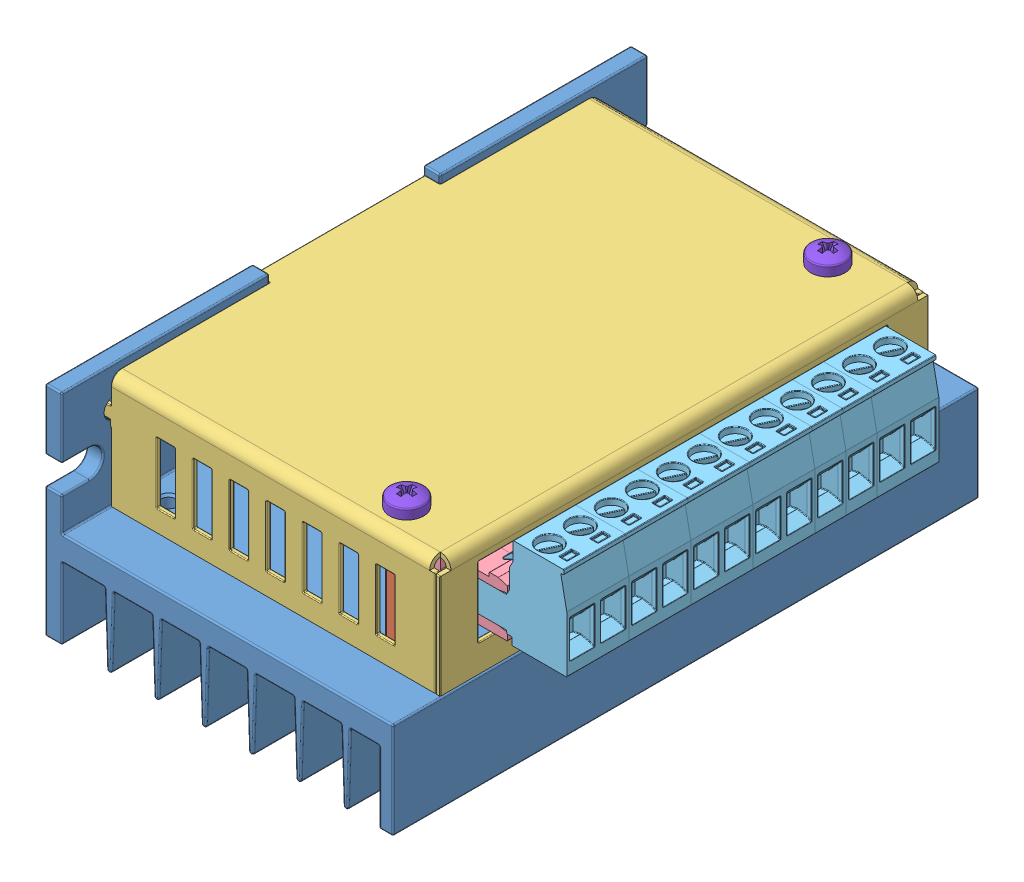
SolidWorks assembly TB6600, configuration Default. Lengths in mm.
Overall size (70.98 37.35 96).
12 component instances, 8 part files, 33 mates.
Components (placement in the parent):
- TB6600 Sink-1: TB6600 Sink [Default] at origin size (57 35.75 96)
- Distance-1: Distance [M3x18] at (43 0 -34.5) size (5 24 4.5)
- Distance-2: Distance [M3x18] at (43 0 34.5) size (5 24 4.5)
- TB6600 Cover-1: TB6600 Cover [Default] at (0 18.75 0) size (56.5 19.75 80)
- Header 200mil-1: Header 200mil [N12] at (48.5 6.85 30.96) size (12 12.2 60.96)
- Plug 200mil-2: Plug 200mil [N2] at (62.83 10.65 25.88) x (-1 0 0) z (0 0 -1) size (18.2 15 10.16)
- Plug 200mil-3: Plug 200mil [N4] at (62.83 10.65 5.56) x (-1 0 0) z (0 0 -1) size (18.2 15 20.32)
- Plug 200mil-4: Plug 200mil [N6] at (62.83 10.65 -24.92) x (-1 0 0) z (0 0 -1) size (18.2 15 30.48)
- LED 3mm Double Stand-1: LED 3mm Double Stand [Default] at (45 5.84 -31) size (11.75 10.16 4.5)
- a6fr-6101-1: a6fr-6101 [Default] at (36.4 6.2 -36.5) x (-1 0 0) z (0 0 -1) size (16.8 13.4 9.9)
- pan head cross recess screw_iso-1: pan head cross recess screw_iso [ISO 7045 - M3 x 4 - Z - 4C] at (43 21.15 -34.5) x (0 -1 0) z (0 0 -1) size (6.35 5.6 5.6)
- pan head cross recess screw_iso-2: pan head cross recess screw_iso [ISO 7045 - M3 x 4 - Z - 4C] at (43 21.15 34.5) x (0 -1 0) z (0 0 -1) size (6.35 5.6 5.6)
Mates (geometry in assembly coordinates):
- Concentric1: concentric aligned: cylinder of TB6600 Sink-1 through (43 0 -34.5) axis (0 1 0) radius 1.25; cylinder of Distance-1 through (43 -6 -34.5) axis (0 1 0) radius 1.5
- Concentric2: concentric aligned: cylinder of TB6600 Sink-1 through (43 0 34.5) axis (0 1 0) radius 1.25; cylinder of Distance-2 through (43 -6 34.5) axis (0 1 0) radius 1.5
- Coincident1: coincident: plane of TB6600 Sink-1 through (0.25 0 48) normal (0 1 0); plane of Distance-1 through (43 0 -34.5) normal (0 -1 0)
- Coincident2: coincident anti-aligned: plane of TB6600 Sink-1 through (0.25 0 48) normal (0 1 0); plane of Distance-2 through (43 0 34.5) normal (0 -1 0)
- Parallel1: parallel aligned: plane of TB6600 Sink-1 through (0 0 0) normal (1 0 0); plane of Distance-1 through (43 0 -34.5) normal (1 0 0)
- Parallel2: parallel aligned: plane of TB6600 Sink-1 through (0 0 0) normal (1 0 0); plane of Distance-2 through (43 0 34.5) normal (1 0 0)
- Concentric3: concentric aligned: cylinder of Distance-2 through (43 18 34.5) axis (0 1 0) radius 1.25; cylinder of TB6600 Cover-1 through (43 18.75 34.5) axis (0 1 0) radius 1.5
- Concentric4: concentric aligned: cylinder of Distance-1 through (43 18 -34.5) axis (0 1 0) radius 1.25; cylinder of TB6600 Cover-1 through (43 18.75 -34.5) axis (0 1 0) radius 1.5
- Coincident3: coincident anti-aligned: plane of Distance-1 through (43 18 -34.5) normal (0 1 0); plane of TB6600 Cover-1 through (53.25 18 40) normal (0 -1 0)
- Concentric5: concentric aligned: cylinder of TB6600 Cover-1 through (43 18.75 -34.5) axis (0 1 0) radius 1.5; cylinder of pan head cross recess screw_iso-1 through (43 46.55 -34.5) axis (0 1 0) radius 1.5
- Concentric6: concentric aligned: cylinder of TB6600 Cover-1 through (43 18.75 34.5) axis (0 1 0) radius 1.5; cylinder of pan head cross recess screw_iso-2 through (43 46.55 34.5) axis (0 1 0) radius 1.5
- Coincident4: coincident anti-aligned: plane of TB6600 Cover-1 through (53.25 18.75 40) normal (0 1 0); plane of pan head cross recess screw_iso-1 through (41.5 18.75 -34.5) normal (0 -1 0)
- Coincident5: coincident anti-aligned: plane of TB6600 Cover-1 through (53.25 18.75 40) normal (0 1 0); plane of pan head cross recess screw_iso-2 through (41.5 18.75 34.5) normal (0 -1 0)
- Parallel3: parallel anti-aligned: plane of TB6600 Sink-1 through (0 0 0) normal (1 0 0); plane of pan head cross recess screw_iso-1 through (43 21.15 -34.5) normal (-1 0 0)
- Parallel4: parallel anti-aligned: plane of TB6600 Sink-1 through (0 0 0) normal (1 0 0); plane of pan head cross recess screw_iso-2 through (43 21.15 34.5) normal (-1 0 0)
- Distance1: distance = 14.5 mm aligned: plane of TB6600 Sink-1 through (0.25 0 48) normal (0 1 0); plane of Header 200mil-1 through (55.5 14.5 28.42) normal (0 1 0)
- Distance2: distance = 14.5 mm aligned: plane of TB6600 Sink-1 through (-0.25 19.75 48) normal (0 0 1); plane of Header 200mil-1 through (48.5 6.85 33.5) normal (0 0 1)
- Distance3: distance = 4.25 mm aligned: plane of TB6600 Sink-1 through (54.25 -0.25 48) normal (1 0 0); plane of Header 200mil-1 through (58.5 6.85 28.42) normal (1 0 0)
- Concentric7: concentric anti-aligned: cylinder of Header 200mil-1 through (49.75 10.65 25.88) axis (1 0 0) radius 1.5; cylinder of Plug 200mil-2 through (51.78 10.65 25.88) axis (-1 0 0) radius 1.5
- Concentric8: concentric anti-aligned: cylinder of Header 200mil-1 through (49.75 10.65 30.96) axis (1 0 0) radius 1.5; cylinder of Plug 200mil-2 through (51.78 10.65 30.96) axis (-1 0 0) radius 1.5
- Concentric9: concentric anti-aligned: cylinder of Header 200mil-1 through (49.75 10.65 20.8) axis (1 0 0) radius 1.5; cylinder of Plug 200mil-3 through (51.78 10.65 20.8) axis (-1 0 0) radius 1.5
- Concentric10: concentric anti-aligned: cylinder of Header 200mil-1 through (49.75 10.65 5.56) axis (1 0 0) radius 1.5; cylinder of Plug 200mil-3 through (51.78 10.65 5.56) axis (-1 0 0) radius 1.5
- Concentric11: concentric anti-aligned: cylinder of Header 200mil-1 through (49.75 10.65 -24.92) axis (1 0 0) radius 1.5; cylinder of Plug 200mil-4 through (51.78 10.65 -24.92) axis (-1 0 0) radius 1.5
- Concentric12: concentric anti-aligned: cylinder of Header 200mil-1 through (49.75 10.65 0.48) axis (1 0 0) radius 1.5; cylinder of Plug 200mil-4 through (51.78 10.65 0.48) axis (-1 0 0) radius 1.5
- Tangent1: tangent anti-aligned: cylinder of Header 200mil-1 through (58.4 13.7347 28.42) axis (0 0 1) radius 0.1; plane of Plug 200mil-2 through (58.33 13.4 23.34) normal (-0.876216 0.481919 0)
- Tangent2: tangent anti-aligned: cylinder of Header 200mil-1 through (58.4 13.7347 18.26) axis (0 0 1) radius 0.1; plane of Plug 200mil-3 through (58.33 13.4 18.26) normal (-0.876216 0.481919 0)
- Tangent3: tangent anti-aligned: cylinder of Header 200mil-1 through (58.4 13.7347 -2.06) axis (0 0 1) radius 0.1; plane of Plug 200mil-4 through (58.33 13.4 -2.06) normal (-0.876216 0.481919 0)
- Coincident6: coincident anti-aligned: plane of TB6600 Cover-1 through (-2.501 16 33.75) normal (0 -1 0); plane of LED 3mm Double Stand-1 through (54 16 -28.75) normal (0 1 0)
- Coincident7: coincident aligned: plane of TB6600 Cover-1 through (54 18.75 0) normal (1 0 0); plane of LED 3mm Double Stand-1 through (54 16 -28.75) normal (1 0 0)
- Coincident8: coincident anti-aligned: plane of TB6600 Cover-1 through (-2.501 16 -33.25) normal (0 0 1); plane of LED 3mm Double Stand-1 through (45 5.84 -33.25) normal (0 0 -1)
- Distance4: distance = 6 mm anti-aligned: plane of a6fr-6101-1 through (19.6 6 -28.25) normal (0 -1 0); plane of TB6600 Sink-1 through (0.25 0 48) normal (0 1 0)
- Distance5: distance = 39.15 mm anti-aligned: plane of a6fr-6101-1 through (36.4 15.375 -35.675) normal (1 0 0); plane of TB6600 Sink-1 through (-2.75 -15.5 48) normal (-1 0 0)
- Distance6: distance = 11.5 mm aligned: plane of TB6600 Sink-1 through (-0.25 19.75 -48) normal (0 0 -1); plane of a6fr-6101-1 through (19.6 15.375 -36.5) normal (0 0 -1)
